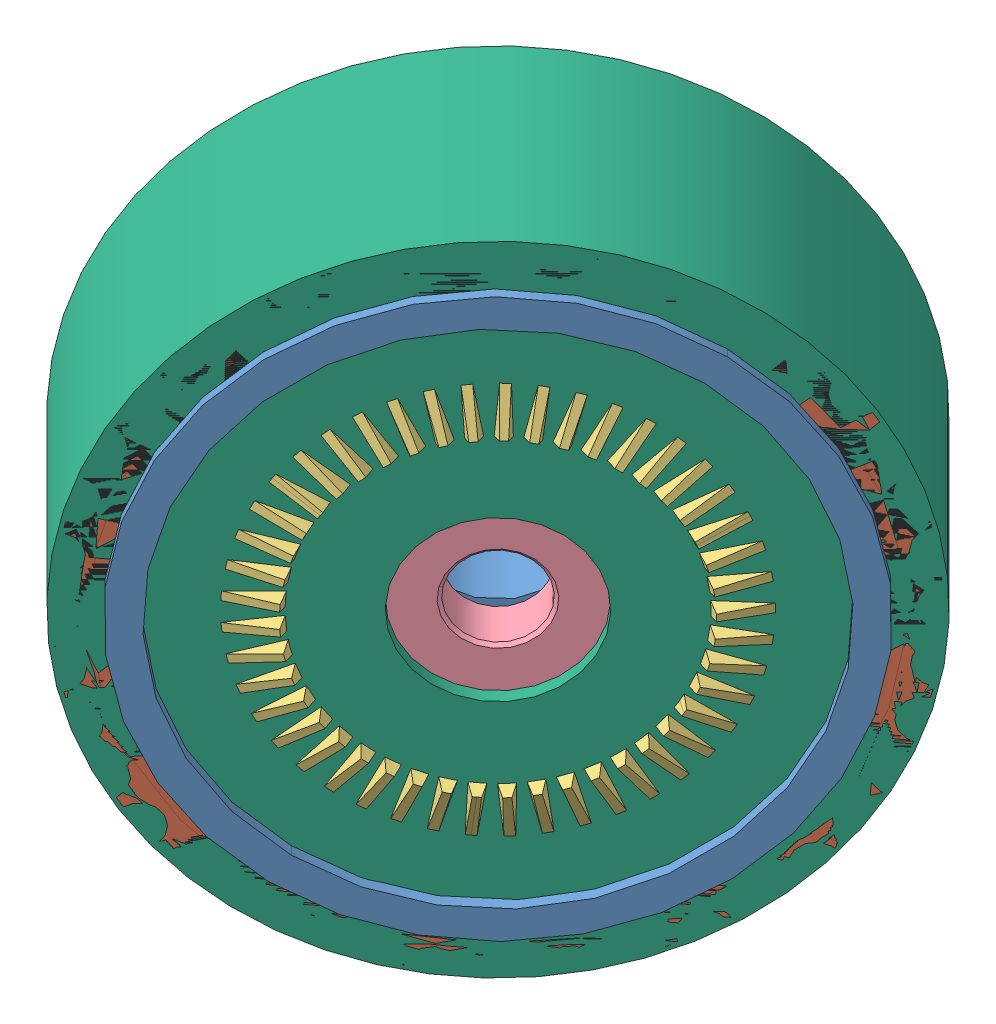
SolidWorks assembly MK4wheel, configuration Default. Lengths in mm.
Overall size (128.67 139.68 128.67).
7 component instances, 6 part files, 2 mates.
Components (placement in the parent):
- MK4 Billet Wheel Assembly.STEP-1: MK4 Billet Wheel Assembly.STEP [Default] at (-66.675 50.7435 -66.675) x (0.707107 0 0.707107) z (0.41117 0.813559 -0.41117) size (42.28 100.13 100.13)
  - Wheel, SDS, Nitrile Tread, 4in X 1.5in, Bearing Bore.STEP-1: Wheel, SDS, Nitrile Tread, 4in X 1.5in, Bearing Bore.STEP [Default] at origin size (42.28 88.9 88.9)
  - Tread, Blue Nitrile 4in X 1.5in.STEP-1: Tread, Blue Nitrile 4in X 1.5in.STEP [Default] at origin size (38.1 100.13 100.13)
- Bevel Gear, 4515.STEP-1: Bevel Gear, 4515.STEP [Default] at (-54.7746 50.7435 -54.7746) x (0.575273 -0.581482 -0.575273) z (-0.41117 -0.813559 0.41117) size (68.38 7.77 68.42)
- Bearing, R8ZZ.STEP-1: Bearing, R8ZZ.STEP [Default] at (-57.5286 50.7435 -57.5286) x (-0.158587 -0.974526 0.158587) z (-0.689094 0.224275 0.689094) size (28.57 7.94 28.57)
- Bearing, R6ZZ.STEP-1: Bearing, R6ZZ.STEP [Default] at (-79.2721 50.7435 -79.2721) x (-0.694824 0.18558 0.694824) z (0.131225 0.982629 -0.131225) size (22.23 7.14 22.23)
- WheelCollision-1: WheelCollision [Rev 1.1] at (-80.1454 50.7435 -80.1454) x (0.706764 -0.031147 -0.706764) z (0.707107 0 0.707107) size (101.6 101.6 38.1)
Mates (geometry in assembly coordinates):
- Concentric1: concentric aligned: cylinder of Bearing, R8ZZ.STEP-1 through (-54.7223 50.7435 -54.7223) axis (-0.707107 0 -0.707107) radius 6.35; cylinder of ColWheel-1 through (-53.2046 50.7435 -53.2046) axis (-0.707107 0 -0.707107) radius 12.7
- Coincident1: coincident aligned: circle of MK4 Billet Wheel Assembly.STEP-1/Tread, Blue Nitrile 4in X 1.5in.STEP-1; plane of ColWheel-1 through (-80.1454 50.7435 -80.1454) normal (-0.707107 0 -0.707107)
